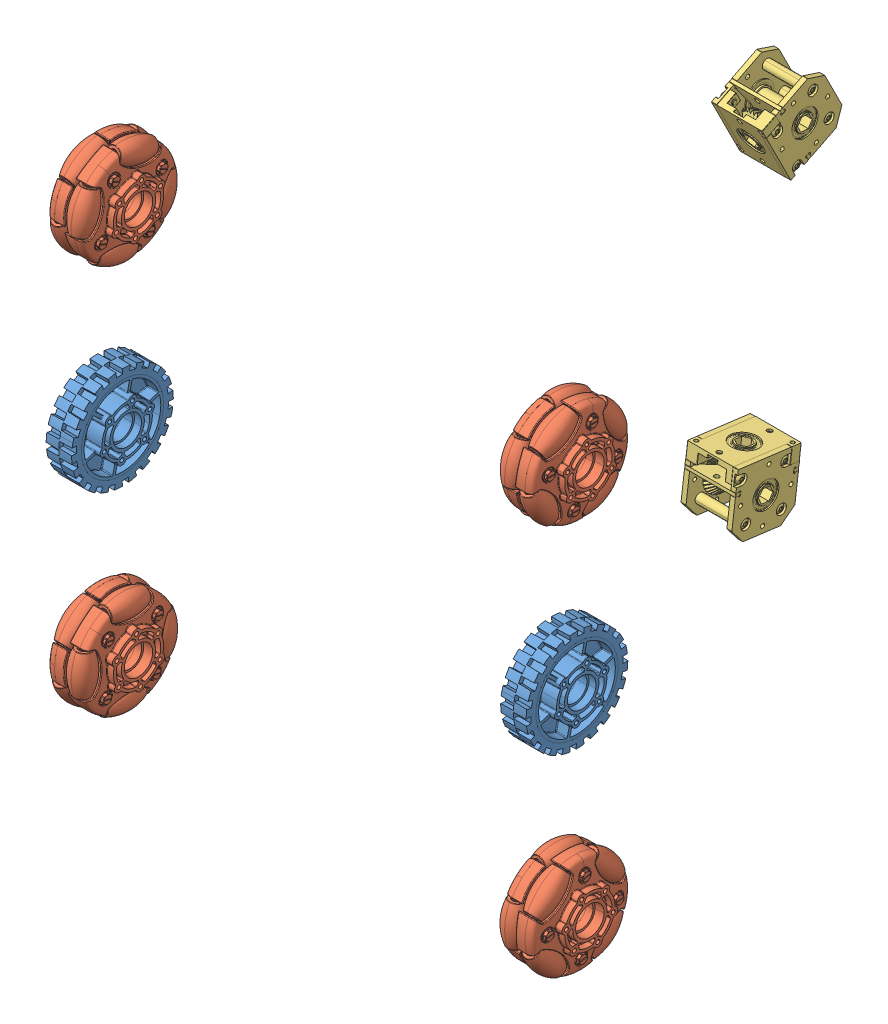
SolidWorks assembly Sponsor-Bot, configuration Default. Lengths in mm.
Overall size (558.8 566.67 589.66).
14 component instances, 6 part files, 22 mates.
Components (placement in the parent):
- Cut-End-Plate-1: Cut-End-Plate [Default] at (-393.7 -283.337 39.37) size (558.8 53.98 84.58)
- Cut-Inside-Plate-1: Cut-Inside-Plate [Default] at (-196.85 406.4 34.925) x (0 -1 0) z (0 0 1) size (558.8 38.1 116.33)
- Cut-Outside-Plate-1: Cut-Outside-Plate [Default] at (-260.35 406.4 34.925) x (0 -1 0) z (0 0 1) size (558.8 22.23 77.72)
- Cut-Inside-Plate-2: Cut-Inside-Plate [Default] at (196.85 -406.4 34.925) x (0 1 0) z (0 0 1) size (558.8 38.1 116.33)
- Cut-Outside-Plate-2: Cut-Outside-Plate [Default] at (260.35 -406.4 34.925) x (0 1 0) z (0 0 1) size (558.8 22.23 77.72)
- Cut-End-Plate-2: Cut-End-Plate [Default] at (393.7 283.337 39.37) x (-1 0 0) z (0 0 1) size (558.8 53.98 84.58)
- am-2256 4 in HiGrip Wheel-1: am-2256 4 in HiGrip Wheel [Default] at (235.0642 3.022 19.5658) x (1 0 0) z (0 -0.221374 -0.975189) size (35.12 101.6 101.6)
- am-3047_4inDuraOmniV2-1: am-3047_4inDuraOmniV2 [Default] at (216.535 -195.0385 15.875) x (0 0.671694 -0.740829) z (1 0 0) size (115.25 115.25 50.88)
- am-3047_4inDuraOmniV2-2: am-3047_4inDuraOmniV2 [Default] at (216.535 195.0385 15.875) x (0 0.499602 -0.866255) z (1 0 0) size (115.25 115.25 50.88)
- am-2256 4 in HiGrip Wheel-3: am-2256 4 in HiGrip Wheel [Default] at (-235.0642 -1.8999 20.6831) x (-1 0 0) z (0 -0.221374 -0.975189) size (35.12 101.6 101.6)
- am-3047_4inDuraOmniV2-5: am-3047_4inDuraOmniV2 [Default] at (-216.535 -195.0385 15.875) x (0 0.671694 -0.740829) z (-1 0 0) size (115.25 115.25 50.88)
- am-3047_4inDuraOmniV2-6: am-3047_4inDuraOmniV2 [Default] at (-216.535 195.0385 15.875) x (0 0.499602 -0.866255) z (-1 0 0) size (115.25 115.25 50.88)
- 90deg gearbox-1: 90deg gearbox [Default] at (-25.4 128.511 -433.0034) x (0 -0.893401 -0.44926) z (1 0 0) size (63.5 63.5 50.8)
- 90deg gearbox-2: 90deg gearbox [Default] at (-25.4 -146.7584 -413.109) x (0 -0.128109 -0.99176) z (-1 0 0) size (63.5 63.5 50.8)
Mates (geometry in assembly coordinates):
- Coincident2: coincident anti-aligned: plane of Cut-End-Plate-1 through (393.7 -229.362 -38.862) normal (0 0 1); plane of Cut-Outside-Plate-1 through (-260.35 -406.4 -38.862) normal (0 0 -1)
- Concentric4: concentric anti-aligned: cylinder of Cut-End-Plate-1 through (-273.05 -266.7 -42.037) axis (0 0 1) radius 2.667; cylinder of Cut-Outside-Plate-1 through (-273.05 -266.7 38.862) axis (0 0 -1) radius 2.667
- Concentric5: concentric aligned: cylinder of Cut-End-Plate-1 through (-273.05 -241.3 -36.957) axis (0 0 -1) radius 2.667; cylinder of Cut-Outside-Plate-1 through (-273.05 -241.3 38.862) axis (0 0 -1) radius 2.667
- Concentric6: concentric anti-aligned: cylinder of Cut-Inside-Plate-1 through (-209.55 -266.7 38.862) axis (0 0 -1) radius 2.667; cylinder of Cut-End-Plate-1 through (-209.55 -266.7 -42.037) axis (0 0 1) radius 2.667
- Coincident5: coincident anti-aligned: plane of Cut-End-Plate-1 through (393.7 -229.362 -38.862) normal (0 0 1); plane of Cut-Inside-Plate-1 through (-196.85 -406.4 -38.862) normal (0 0 -1)
- Parallel3: parallel anti-aligned: plane of Cut-Inside-Plate-1 through (-196.85 406.4 -34.925) normal (-1 0 0); plane of Cut-Outside-Plate-1 through (-257.175 406.4 -34.925) normal (1 0 0)
- Distance2: distance = 279.4 mm: plane of assembly through (0 0 0) normal (1 0 0); plane of assembly; plane of Cut-End-Plate-1 through (-279.4 -283.337 39.37) normal (-1 0 0)
- Distance3: distance = 279.4 mm: plane of assembly through (0 0 0) normal (0 1 0); plane of assembly; plane of Cut-Outside-Plate-1 through (-260.35 -279.4 34.925) normal (0 -1 0)
- Distance4: distance = 38.862 mm: plane of assembly through (0 0 0) normal (0 0 1); plane of assembly; plane of Cut-Outside-Plate-1 through (-260.35 -406.4 38.862) normal (0 0 1)
- Concentric7: concentric anti-aligned: cylinder of Cut-Outside-Plate-2 through (260.35 0 17.653) axis (-1 0 0) radius 14.2875; cylinder of am-2256 4 in HiGrip Wheel-1 through (209.55 0 17.653) axis (1 0 0) radius 12.2174
- Distance5: distance = 12.7 mm anti-aligned: plane of am-2256 4 in HiGrip Wheel-1 through (244.475 0 17.653) normal (1 0 0); plane of Cut-Outside-Plate-2 through (257.175 -406.4 -34.925) normal (-1 0 0)
- Concentric8: concentric anti-aligned: cylinder of Cut-Outside-Plate-2 through (368.301 -195.0385 15.875) axis (-1 0 0) radius 4.826; cylinder of am-3047_4inDuraOmniV2-1 through (204.0339 -195.0385 15.875) axis (1 0 0) radius 12.2428
- Distance6: distance = 6.35 mm anti-aligned: plane of Cut-Outside-Plate-2 through (257.175 -406.4 -34.925) normal (-1 0 0); plane of am-3047_4inDuraOmniV2-1 through (250.825 -195.0385 15.875) normal (1 0 0)
- Concentric9: concentric anti-aligned: cylinder of Cut-Outside-Plate-2 through (368.301 195.0385 15.875) axis (-1 0 0) radius 4.826; cylinder of am-3047_4inDuraOmniV2-2 through (215.8999 195.0385 15.875) axis (1 0 0) radius 12.2428
- Distance7: distance = 6.35 mm anti-aligned: plane of am-3047_4inDuraOmniV2-2 through (250.825 195.0385 15.875) normal (1 0 0); plane of Cut-Outside-Plate-2 through (257.175 -406.4 -34.925) normal (-1 0 0)
- Coincident12: coincident anti-aligned: plane of Cut-End-Plate-1 through (393.7 -229.362 -42.037) normal (0 0 -1); plane of Rev Extrusion-1 through (-209.409 282.0644 -42.037) normal (0 0 1)
- Concentric10: concentric anti-aligned: cylinder of 90deg gearbox-1 through (-50.8 136.9346 -449.7547) axis (-1 0 0) radius 8.495
- Parallel4: parallel: plane of 90deg gearbox-1 through (0 108.5691 -464.0187) normal (0 -0.893401 -0.44926)
- Coincident14: coincident aligned: plane of 90deg gearbox-1 through (0 136.9346 -449.7547) normal (1 0 0)
- Coincident15: coincident aligned: plane of 90deg gearbox-1 through (0 136.9346 -449.7547) normal (1 0 0); plane of 90deg gearbox-2 through (0 -165.3539 -410.707) normal (1 0 0)
- Concentric11: concentric aligned: cylinder of 90deg gearbox-2 through (0 -165.3539 -410.707) axis (1 0 0) radius 8.495
- Parallel5: parallel: plane of 90deg gearbox-2 through (0 -169.4213 -442.1954) normal (0 -0.128109 -0.99176)
